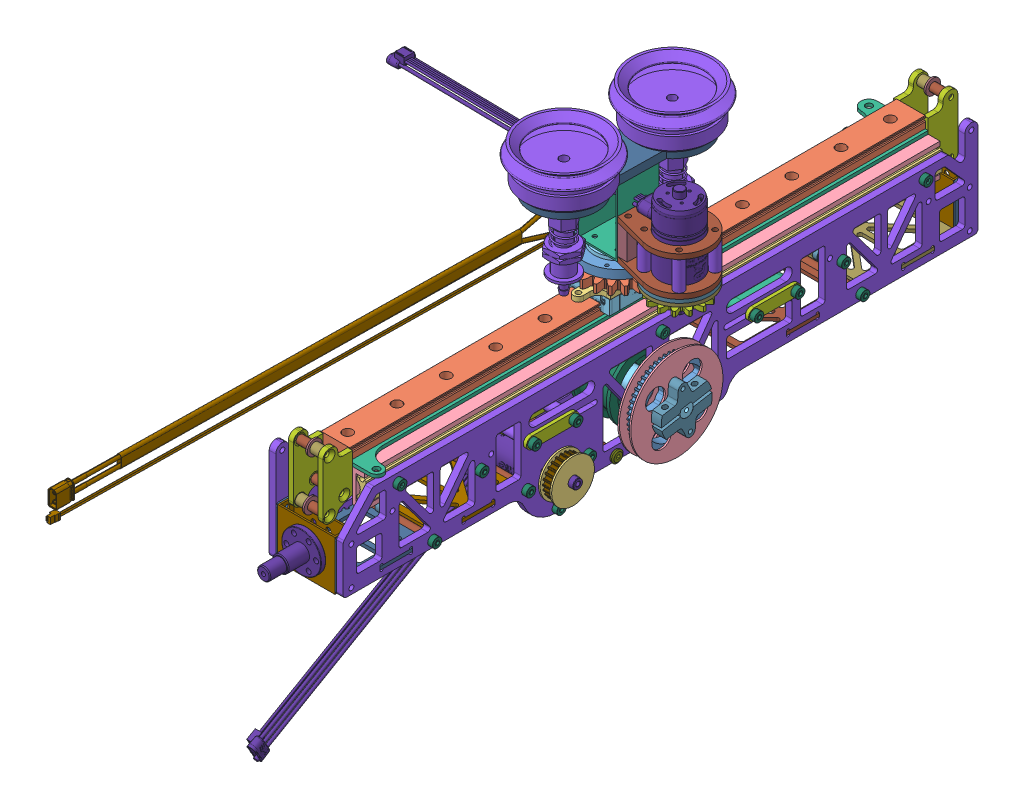
SolidWorks assembly 取矿横移总装, configuration 默认. Lengths in mm.
Overall size (203.34 276.76 526.28).
149 component instances, 51 part files, 3 mates.
Components (placement in the parent):
- 横移总装2.0-1: 横移总装2.0 [默认] at origin size (67.7 199.63 415.26)
  - 20x20x1铝方管-1: 20x20x1铝方管 [默认] at (0 2.5 0.2898) size (15 15 350)
  - 上银直线导轨线性滑轨MGW-C╱MGW-H[MGW9C2R355EZACHCI]_2-1: 上银直线导轨线性滑轨MGW-C╱MGW-H[MGW9C2R355EZACHCI]_2 [横移] at (0 14.9 0.2898) size (18 7 350)
  - 铝合金抽屉滑轨_350-1: 铝合金抽屉滑轨_350 [默认] at (12.9 0 0) x (0 0 -1) z (-1 0 0) size (350.29 20 8) (flexible)
    - 铝合金抽屉滑轨内侧_350-1: 铝合金抽屉滑轨内侧_350 [默认] at origin size (350 12 5.6)
    - 铝合金抽屉滑轨外侧_350-1: 铝合金抽屉滑轨外侧_350 [默认] at (-0.2898 0 2.4) size (350 20 7.2)
  - 铝合金抽屉滑轨_350-2: 铝合金抽屉滑轨_350 [默认] at (-12.9 0 0) x (0 0 -1) z (1 0 0) size (350.29 20 8) (flexible)
    - 铝合金抽屉滑轨内侧_350-1: 铝合金抽屉滑轨内侧_350 [默认] at origin size (350 12 5.6)
    - 铝合金抽屉滑轨外侧_350-1: 铝合金抽屉滑轨外侧_350 [默认] at (-0.2898 0 2.4) size (350 20 7.2)
  - 上银直线导轨线性滑轨MGW-C╱MGW-H[MGW9C2R355EZACHCI]_1-1: 上银直线导轨线性滑轨MGW-C╱MGW-H[MGW9C2R355EZACHCI]_1 [MGW9C] at (0 14.9 3.3555) size (30 9.1 39.49)
  - 滑轨安装板-1: 滑轨安装板 [默认] at (0 10 0.2898) x (0 0 -1) z (0 1 0) size (350 50.5 2)
  - 转点安装板1-1: 转点安装板1 [默认] at (7.5 2.5 160.2898) x (0 0 -1) z (1 0 0) size (48 39.5 3)
  - 转点安装板1-2: 转点安装板1 [默认] at (-10.5 2.5 160.2898) x (0 0 -1) z (1 0 0) size (48 39.5 3)
  - 转点安装板1-3: 转点安装板1 [默认] at (10.5 2.5 -159.7102) x (0 0 1) z (-1 0 0) size (48 39.5 3)
  - 转点安装板1-4: 转点安装板1 [默认] at (-7.5 2.5 -159.7102) x (0 0 1) z (-1 0 0) size (48 39.5 3)
  - 安装固定板-2: 安装固定板 [非2006安装板] at (-22.5 -20 0) x (0 0 -1) z (1 0 0) size (386 79.31 4)
  - 35x10x1铝方管-1: 35x10x1铝方管 [默认] at (0 -30 188) x (1 0 0) z (0 -1 0) size (35 10 30)
  - 垫板-1: 垫板 [默认] at (-18 -30 188) x (0 0 1) z (-1 0 0) size (10 30 1)
  - 垫板-2: 垫板 [默认] at (18 -30 188) x (0 0 1) z (-1 0 0) size (10 30 1)
  - 35x10x1铝方管-2: 35x10x1铝方管 [默认] at (0 -30 -188) x (1 0 0) z (0 -1 0) size (35 10 30)
  - 垫板-3: 垫板 [默认] at (-18 -30 -188) x (0 0 1) z (-1 0 0) size (10 30 1)
  - 垫板-4: 垫板 [默认] at (18 -30 -188) x (0 0 1) z (-1 0 0) size (10 30 1)
  - 鸿康明铝柱-1: 鸿康明铝柱 [M3*8] at (-3.5 22.5 189.2898) x (1 0 0) z (0 -0.954265 0.298963) size (8 5 5)
  - 粉末冶金铜套-1: 粉末冶金铜套 [默认] at (4.5 22.5 189.2898) x (0 0.169784 0.985481) z (-1 0 0) size (6 6 6)
  - 3x9x1垫片-1: 3x9x1垫片 [默认] at (1 22.5 189.2898) x (0 -0.61264 -0.790362) z (1 0 0) size (9 9 1)
  - 鸿康明铝柱-2: 鸿康明铝柱 [M3*8] at (-3.5 -2.5 180.2898) x (1 0 0) z (0 -0.617564 0.786521) size (8 5 5)
  - 粉末冶金铜套-2: 粉末冶金铜套 [默认] at (4.5 -2.5 180.2898) x (0 -0.015386 0.999882) z (-1 0 0) size (6 6 6)
  - 3x9x1垫片-2: 3x9x1垫片 [默认] at (1 -2.5 180.2898) x (0 -0.61264 -0.790362) z (1 0 0) size (9 9 1)
  - 粉末冶金铜套-3: 粉末冶金铜套 [默认] at (-4.5 -9 189.2898) x (0 -0.015317 0.999883) z (-1 0 0) size (6 6 6)
  - 鸿康明铝柱-3: 鸿康明铝柱 [M3*8] at (3.5 -9 189.2898) x (1 0 0) z (0 -0.94021 0.340594) size (8 5 5)
  - 3x9x1垫片-3: 3x9x1垫片 [默认] at (-1 -9 189.2898) x (0 -0.634328 -0.773064) z (1 0 0) size (9 9 1)
  - 鸿康明铝柱-4: 鸿康明铝柱 [M3*8] at (3.5 22.5 -188.7102) x (1 0 0) z (0 -0.954265 0.298963) size (8 5 5)
  - 粉末冶金铜套-4: 粉末冶金铜套 [默认] at (-4.5 22.5 -188.7102) x (0 0.169784 0.985481) z (-1 0 0) size (6 6 6)
  - 3x9x1垫片-4: 3x9x1垫片 [默认] at (-1 22.5 -188.7102) x (0 -0.708763 -0.705447) z (1 0 0) size (9 9 1)
  - 鸿康明铝柱-5: 鸿康明铝柱 [M3*8] at (3.5 -2.5 -179.7102) x (1 0 0) z (0 -0.919061 0.394116) size (8 5 5)
  - 粉末冶金铜套-5: 粉末冶金铜套 [默认] at (-4.5 -2.5 -179.7102) x (0 0.138586 0.99035) z (-1 0 0) size (6 6 6)
  - 3x9x1垫片-5: 3x9x1垫片 [默认] at (-1 -2.5 -179.7102) x (0 -0.708763 -0.705447) z (1 0 0) size (9 9 1)
  - 鸿康明铝柱-6: 鸿康明铝柱 [M3*8] at (-3.5 -9 -188.7102) x (1 0 0) z (0 -0.453676 0.891166) size (8 5 5)
  - 3x9x1垫片-6: 3x9x1垫片 [默认] at (1 -9 -188.7102) x (0 -0.708763 -0.705447) z (1 0 0) size (9 9 1)
  - 粉末冶金铜套-6: 粉末冶金铜套 [默认] at (4.5 -9 -188.7102) x (0 0.138586 0.99035) z (-1 0 0) size (6 6 6)
  - 深沟球轴承-1: 深沟球轴承 [3x7x3] at (15.2 -13.5 163) x (0 -0.844681 -0.53527) z (0 -0.53527 0.844681) size (7 3 7)
  - 深沟球轴承-2: 深沟球轴承 [3x7x3] at (15.2 0.4813 104.6517) x (0 -0.771668 0.636026) z (0 0.636026 0.771668) size (7 3 7)
  - 深沟球轴承-3: 深沟球轴承 [3x7x3] at (15.2 -13.5 -103) x (0 -0.533975 -0.845501) z (0 -0.845501 0.533975) size (7 3 7)
  - 深沟球轴承-4: 深沟球轴承 [3x7x3] at (15.2 -13.5 -163) x (0 0.004458 -0.99999) z (0 -0.99999 -0.004458) size (7 3 7)
  - 深沟球轴承-5: 深沟球轴承 [3x7x3] at (-18.2 -13.5 163) x (0 -0.963854 -0.266431) z (0 -0.266431 0.963854) size (7 3 7)
  - 深沟球轴承-6: 深沟球轴承 [3x7x3] at (-18.2 -13.5 103) x (0 0.996588 0.082533) z (0 0.082533 -0.996588) size (7 3 7)
  - 深沟球轴承-7: 深沟球轴承 [3x7x3] at (-18.2 -13.5 -103) x (0 -0.057804 -0.998328) z (0 -0.998328 0.057804) size (7 3 7)
  - 深沟球轴承-8: 深沟球轴承 [3x7x3] at (-18.2 -13.5 -163) x (0 -0.915157 -0.403098) z (0 -0.403098 0.915157) size (7 3 7)
  - 铰轮1.0-1: 铰轮1.0 [默认] at (0 -34 0) x (0 0.984367 0.176128) z (0 -0.176128 0.984367) size (41 24 41)
  - 法兰轴承-1: 法兰轴承 [10*19*5-1] at (17.5 -34 0) x (0 -0.704143 0.710058) z (0 0.710058 0.704143) size (21 5 21)
  - RoboMaster M2006 P36直流无刷减速电机-1: RoboMaster M2006 P36直流无刷减速电机 [默认] at (-11.3952 -31.5927 46.0167) x (0 -0.258819 -0.965926) z (-1 0 0) size (140.17 141.41 64.8)
  - 安装固定板-3: 安装固定板 [2006安装板] at (18.5 -20 0) x (0 0 -1) z (1 0 0) size (386 79.31 4)
  - 小带轮3Mx25-1: 小带轮3Mx25 [默认] at (25.4 -42.8 63.1397) x (1 0 0) z (0 -0.934457 -0.356076) size (6 23.05 23.09)
  - 大带轮3Mx50-1: 大带轮3Mx50 [默认] at (25.4 -34 0) x (1 0 0) z (0 0.986511 0.163695) size (6 46.93 46.99)
  - 推力球轴承-1: 推力球轴承 [F6-12M 6*12*4] at (24.4 -42.8 63.1397) x (0 0.637207 0.770693) z (0 -0.770693 0.637207) size (12 4 12)
  - 小带轮挡边-1: 小带轮挡边 [默认] at (25.4 -42.8 63.1397) x (0 0.491726 0.87075) z (-1 0 0) size (26 26 1)
  - 小带轮挡边-2: 小带轮挡边 [默认] at (32.4 -42.8 63.1397) x (0 0.997033 0.076981) z (-1 0 0) size (26 26 1)
  - 大带轮挡边-1: 大带轮挡边 [默认] at (32.4 -34 0) x (0 -0.163695 0.986511) z (-1 0 0) size (56 56 1)
  - 大带轮挡边-2: 大带轮挡边 [默认] at (25.4 -34 0) x (0 -0.163695 0.986511) z (-1 0 0) size (56 56 1)
  - 法兰轴承-2: 法兰轴承 [10*19*5-1] at (-17.5 -34 0) x (0 0.968123 0.250476) z (0 -0.250476 0.968123) size (21 5 21)
  - 传动轴-1: 传动轴 [默认] at (-22.5 -34 0) x (0 -0.984367 -0.176128) z (-1 0 0) size (24 24 60.8)
  - 鸿康明铝柱-7: 鸿康明铝柱 [M3*37] at (0 -18 110) size (37 5 5)
  - 鸿康明铝柱-8: 鸿康明铝柱 [M3*37] at (0 -18 -110) size (37 5 5)
  - 槽轮安装件-1: 槽轮安装件 [默认] at (-5 -18 67.5) x (0 0 1) z (0 1 0) size (32 23 7)
  - 槽轮安装件-2: 槽轮安装件 [默认] at (5 -18 -67.5) x (0 0 -1) z (0 1 0) size (32 23 7)
  - 垫片安装-1: 垫片安装 [默认] at (17.5 -18 -67.5) x (0 0 -1) z (1 0 0) size (32 7 2)
  - 垫片安装-2: 垫片安装 [默认] at (-7.5 -18 -67.5) x (0 0 -1) z (1 0 0) size (32 7 2)
  - 垫片安装-3: 垫片安装 [默认] at (-23.5 -18 -67.5) x (0 0 -1) z (1 0 0) size (32 7 2)
  - 304不锈钢接线柱-1: 304不锈钢接线柱 [M3*10-6] at (-13.5 -18 -80) x (0 0.392513 0.919746) z (-1 0 0) size (6 6 10)
  - 304不锈钢接线柱-2: 304不锈钢接线柱 [M3*10-6] at (-13.5 -18 -55) x (0 0.520007 0.854162) z (-1 0 0) size (6 6 10)
  - 垫片安装-4: 垫片安装 [默认] at (23.5 -18 -67.5) x (0 0 -1) z (1 0 0) size (32 7 2)
  - 垫片安装-5: 垫片安装 [默认] at (-17.5 -18 67.5) x (0 0 -1) z (1 0 0) size (32 7 2)
  - 垫片安装-6: 垫片安装 [默认] at (7.5 -18 67.5) x (0 0 -1) z (1 0 0) size (32 7 2)
  - 垫片安装-7: 垫片安装 [默认] at (23.5 -18 67.5) x (0 0 -1) z (1 0 0) size (32 7 2)
  - 垫片安装-8: 垫片安装 [默认] at (-23.5 -18 67.5) x (0 0 -1) z (1 0 0) size (32 7 2)
  - 304不锈钢接线柱-3: 304不锈钢接线柱 [M3*10-6] at (13.5 -18 80) x (0 0.51626 0.856432) z (-1 0 0) size (6 6 10)
  - 304不锈钢接线柱-4: 304不锈钢接线柱 [M3*10-6] at (13.5 -18 55) x (0 0.48843 0.872603) z (-1 0 0) size (6 6 10)
  - 鸿康明铝柱-9: 鸿康明铝柱 [M3*37] at (0 -41 138.7695) size (37 5 5)
  - 鸿康明铝柱-10: 鸿康明铝柱 [M3*37] at (0 -42.8 81.6519) size (37 5 5)
  - 鸿康明铝柱-11: 鸿康明铝柱 [M3*37] at (0 -61.3122 63.1397) size (37 5 5)
  - 鸿康明铝柱-12: 鸿康明铝柱 [M3*37] at (0 -42.8 44.6275) size (37 5 5)
  - 鸿康明铝柱-13: 鸿康明铝柱 [M3*37] at (0 -52 27.5) size (37 5 5)
  - 鸿康明铝柱-14: 鸿康明铝柱 [M3*37] at (0 -52 -27.5) size (37 5 5)
  - 鸿康明铝柱-16: 鸿康明铝柱 [M3*37] at (0 -41 -121.5) x (1 0 0) z (0 -0.672533 0.740067) size (37 5 5)
  - 加强板1-1: 加强板1 [默认] at (0 -39 110.5695) x (0 0 -1) z (0 -1 0) size (50 45 2)
  - 加强板2-1: 加强板2 [默认] at (0 -41 161.9695) x (1 0 0) z (0 1 0) size (45 40 2)
  - 加强板3-1: 加强板3 [默认] at (0 -41 -85.8) x (0 0 1) z (-1 0 0) size (65 2 45)
  - 加强板4-1: 加强板4 [默认] at (0 -41 -153.2) x (0 0 1) z (-1 0 0) size (57 2 45)
  - 2006D型孔联轴器-1: 2006D型孔联轴器 [默认] at (35.4 -42.8 63.1397) x (0 0.844273 0.535914) z (-1 0 0) size (19.05 22 6) (hidden)
  - V型轴承623zz-1: V型轴承623zz [默认] at (4 -18 55) x (1 0 0) z (0 -0.119134 0.992878) size (3.8 12 12)
  - V型轴承623zz-2: V型轴承623zz [默认] at (-4 -18 -55) x (1 0 0) z (0 -0.119134 0.992878) size (3.8 12 12)
  - 夹紧连轴器-1: 夹紧连轴器 [默认] at (35.4 -34 0) x (0 0.176128 -0.984367) z (1 0 0) size (30.94 31 6)
  - 12.9级圆柱头螺钉-1: 12.9级圆柱头螺钉 [M3*10] at (25.5 -41 138.7695) x (0 -0.265301 -0.964166) z (1 0 0) size (5.68 5.68 13)
  - 12.9级圆柱头螺钉-2: 12.9级圆柱头螺钉 [M3*10] at (25.5 -18 110) x (0 -0.265301 -0.964166) z (1 0 0) size (5.68 5.68 13)
  - 12.9级圆柱头螺钉-3: 12.9级圆柱头螺钉 [M3*10] at (25.5 -42.8 81.6519) x (0 -0.265301 -0.964166) z (1 0 0) size (5.68 5.68 13)
  - 12.9级圆柱头螺钉-4: 12.9级圆柱头螺钉 [M3*10] at (27.5 -18 80) x (0 -0.265301 -0.964166) z (1 0 0) size (5.68 5.68 13)
  - 12.9级圆柱头螺钉-5: 12.9级圆柱头螺钉 [M3*10] at (27.5 -18 55) x (0 -0.265301 -0.964166) z (1 0 0) size (5.68 5.68 13)
  - 12.9级圆柱头螺钉-6: 12.9级圆柱头螺钉 [M3*10] at (25.5 -61.3122 63.1397) x (0 -0.265301 -0.964166) z (1 0 0) size (5.68 5.68 13)
  - 12.9级圆柱头螺钉-8: 12.9级圆柱头螺钉 [M3*10] at (25.5 -52 -27.5) x (0 -0.265301 -0.964166) z (1 0 0) size (5.68 5.68 13)
  - 12.9级圆柱头螺钉-9: 12.9级圆柱头螺钉 [M3*10] at (27.5 -18 -55) x (0 -0.265301 -0.964166) z (1 0 0) size (5.68 5.68 13)
  - 12.9级圆柱头螺钉-10: 12.9级圆柱头螺钉 [M3*10] at (27.5 -18 -80) x (0 -0.265301 -0.964166) z (1 0 0) size (5.68 5.68 13)
  - 12.9级圆柱头螺钉-11: 12.9级圆柱头螺钉 [M3*10] at (25.5 -18 -110) x (0 -0.265301 -0.964166) z (1 0 0) size (5.68 5.68 13)
  - 12.9级圆柱头螺钉-12: 12.9级圆柱头螺钉 [M3*10] at (25.5 -41 -121.5) x (0 -0.265301 -0.964166) z (1 0 0) size (5.68 5.68 13)
  - 12.9级圆柱头螺钉-13: 12.9级圆柱头螺钉 [M3*10] at (-25.5 -41 -121.5) x (0 -0.999995 -0.003259) z (-1 0 0) size (5.68 5.68 13)
  - 12.9级圆柱头螺钉-14: 12.9级圆柱头螺钉 [M3*10] at (-25.5 -18 -110) x (0 -0.999995 -0.003259) z (-1 0 0) size (5.68 5.68 13)
  - 12.9级圆柱头螺钉-15: 12.9级圆柱头螺钉 [M3*10] at (-27.5 -18 -80) x (0 -0.999995 -0.003259) z (-1 0 0) size (5.68 5.68 13)
  - 12.9级圆柱头螺钉-16: 12.9级圆柱头螺钉 [M3*10] at (-27.5 -18 -55) x (0 -0.999995 -0.003259) z (-1 0 0) size (5.68 5.68 13)
  - 12.9级圆柱头螺钉-17: 12.9级圆柱头螺钉 [M3*10] at (-25.5 -52 -27.5) x (0 -0.999995 -0.003259) z (-1 0 0) size (5.68 5.68 13)
  - 12.9级圆柱头螺钉-18: 12.9级圆柱头螺钉 [M3*10] at (-25.5 -52 27.5) x (0 -0.999995 -0.003259) z (-1 0 0) size (5.68 5.68 13)
  - 12.9级圆柱头螺钉-19: 12.9级圆柱头螺钉 [M3*10] at (-25.5 -42.8 44.6275) x (0 -0.999995 -0.003259) z (-1 0 0) size (5.68 5.68 13)
  - 12.9级圆柱头螺钉-20: 12.9级圆柱头螺钉 [M3*10] at (-27.5 -18 55) x (0 -0.999995 -0.003259) z (-1 0 0) size (5.68 5.68 13)
  - 12.9级圆柱头螺钉-21: 12.9级圆柱头螺钉 [M3*10] at (-27.5 -18 80) x (0 -0.999995 -0.003259) z (-1 0 0) size (5.68 5.68 13)
  - 12.9级圆柱头螺钉-22: 12.9级圆柱头螺钉 [M3*10] at (-25.5 -61.3122 63.1397) x (0 -0.999995 -0.003259) z (-1 0 0) size (5.68 5.68 13)
  - 12.9级圆柱头螺钉-23: 12.9级圆柱头螺钉 [M3*10] at (-25.5 -42.8 81.6519) x (0 -0.999995 -0.003259) z (-1 0 0) size (5.68 5.68 13)
  - 12.9级圆柱头螺钉-24: 12.9级圆柱头螺钉 [M3*10] at (-25.5 -18 110) x (0 -0.999995 -0.003259) z (-1 0 0) size (5.68 5.68 13)
  - 12.9级圆柱头螺钉-25: 12.9级圆柱头螺钉 [M3*10] at (-25.5 -41 138.7695) x (0 -0.999995 -0.003259) z (-1 0 0) size (5.68 5.68 13)
  - 12.9级圆柱头螺钉-26: 12.9级圆柱头螺钉 [M3*8] at (-25.5 0 160) x (0 -0.999995 -0.003259) z (-1 0 0) size (5.68 5.68 11)
  - 12.9级圆柱头螺钉-27: 12.9级圆柱头螺钉 [M3*8] at (-25.5 0 0) x (0 -0.999995 -0.003259) z (-1 0 0) size (5.68 5.68 11)
  - 12.9级圆柱头螺钉-28: 12.9级圆柱头螺钉 [M3*8] at (-25.5 0 -160) x (0 -0.999995 -0.003259) z (-1 0 0) size (5.68 5.68 11)
  - 12.9级圆柱头螺钉-29: 12.9级圆柱头螺钉 [M3*8] at (25.5 0 -160) x (0 -0.774925 -0.632053) z (1 0 0) size (5.68 5.68 11)
  - 12.9级圆柱头螺钉-30: 12.9级圆柱头螺钉 [M3*8] at (25.5 0 0) x (0 -0.774925 -0.632053) z (1 0 0) size (5.68 5.68 11)
  - 12.9级圆柱头螺钉-31: 12.9级圆柱头螺钉 [M3*8] at (25.5 0 160) x (0 -0.774925 -0.632053) z (1 0 0) size (5.68 5.68 11)
  - 304不锈钢平头倒边螺丝-1: 304不锈钢平头倒边螺丝 [M3*10] at (24.3 -52 27.5) x (0 0.904522 -0.426427) z (1 0 0) size (7 7 11.8)
  - 12.9级圆柱头螺钉-32: 12.9级圆柱头螺钉 [M3*10] at (25.5 -42.8 44.6275) x (0 -0.265301 -0.964166) z (1 0 0) size (5.68 5.68 13)
  - 转点法兰-1: 转点法兰 [默认] at (0 -30 193) x (0.866025 0.5 0) z (0 0 1) size (24 24 26)
- 吸盘总装-1: 吸盘总装 [默认] at (0 34 3.3555) x (-1 0 0) z (0 1 0) size (203.34 428.51 86.1)
  - 6750zz-1: 6750zz [默认] at origin size (32 32 4)
  - 轴承外圈固定-1: 轴承外圈固定 [默认] at (0 0 0.03) x (0 -1 0) z (0 0 1) size (42 42 5.34)
  - 圆柱齿轮24×2-1: 圆柱齿轮24×2 [默认] at (0 0 -4.5) size (51.72 51.72 5)
  - 拉线安装版-1: 拉线安装版 [默认] at (0 0 -10) x (0 1 0) z (0 0 1) size (63.3 30 3)
  - 内圈分离铝件-1: 内圈分离铝件 [默认] at (0 0 1.95) x (-0.717753 -0.696298 0) z (0 0 -1) size (28 28 5.15)
  - 内圈压板-1: 内圈压板 [默认] at (0 0 2) x (0.717753 0.696298 0) z (0 0 1) size (28 28 3)
  - 20x40x1铝方管-2: 20x40x1铝方管 [默认] at (0 0 25) x (-0.999885 0.015171 0) z (0.015171 0.999885 0) size (25 40 25)
  - RoboMaster M2006 P36直流无刷减速电机-1: RoboMaster M2006 P36直流无刷减速电机 [默认] at (-58.4085 2.0306 32.7952) x (-0.717753 -0.696298 0) z (0 0 1) size (140.17 141.41 64.8)
  - 圆柱齿轮14×2-1: 圆柱齿轮14×2 [默认] at (-37.9956 0.5765 -4.5) x (-0.882361 0.470573 0) z (0 0 1) size (32 31.46 3)
  - 推力球轴承-1: 推力球轴承 [F6-12M 6*12*4] at (-37.9956 0.5765 -3) x (0.191226 -0.981546 0) z (-0.981546 -0.191226 0) size (12 4 12)
  - 吸盘-1: 吸盘 [PJTS-50-6-N] at (-0.493 -32.4963 72) x (-0.999885 0.015171 0) z (-0.015171 -0.999885 0) size (54.83 80 54.83)
  - 吸盘-2: 吸盘 [PJTS-50-6-N] at (0.493 32.4963 72) x (0.996645 0.081841 0) z (-0.081841 0.996645 0) size (54.83 80 54.83)
  - C610无刷电机调速器-1: C610无刷电机调速器 [默认] at (16.0987 6.3023 -120.7197) x (0 0 -1) z (0.999885 -0.015171 0) size (22.14 353.32 7.25)
  - 吸盘固定板2-1: 吸盘固定板2 [默认] at (0 0 45) x (0.015171 0.999885 0) z (0 0 1) size (105 40 5)
  - 2006电机紧固板-1: 2006电机紧固板 [默认] at (-37.9956 0.5765 8) x (0.999885 -0.015171 0) z (0 0 -1) size (43.75 36.5 3)
  - 2006电机安装板-1: 2006电机安装板 [默认] at (-37.9956 0.5765 0.9) x (-0.999885 0.015171 0) z (0 0 1) size (35.09 36.5 2)
  - 2006电机紧固板-2: 2006电机紧固板 [默认] at (-37.9956 0.5765 29) x (0.999885 -0.015171 0) z (0 0 -1) size (43.75 36.5 3)
  - 304不锈钢接线柱-1: 304不锈钢接线柱 [M3*18-6] at (-48.9414 -10.0421 17) size (6 6 18)
  - 304不锈钢接线柱-2: 304不锈钢接线柱 [M3*18-6] at (-48.6142 11.5222 17) x (-0.15981 -0.987148 0) z (0 0 1) size (6 6 18)
  - 304不锈钢接线柱-3: 304不锈钢接线柱 [M3*18-6] at (-27.0499 11.195 17) size (6 6 18)
  - 304不锈钢接线柱-4: 304不锈钢接线柱 [M3*18-6] at (-27.3771 -10.3692 17) size (6 6 18)
  - 安装铝件-1: 安装铝件 [默认] at (-15.4982 0.2351 17) x (-0.015171 -0.999885 0) z (0.999885 -0.015171 0) size (25 18 6)
  - 2006电机安装垫块-1: 2006电机安装垫块 [默认] at (-37.9956 0.5765 3.95) x (-0.999885 0.015171 0) z (0 0 1) size (35.09 36.5 2.1)
Mates (geometry in assembly coordinates):
- 重合1: coincident anti-aligned: plane of 横移总装2.0-1/上银直线导轨线性滑轨MGW-C╱MGW-H[MGW9C2R355EZACHCI]_1-1 through (-15 24 17.1055) normal (0 1 0); plane of 吸盘总装-1/拉线安装版-1 through (0 24 3.3555) normal (0 -1 0)
- 宽度1: width anti-aligned: plane of 吸盘总装-1/拉线安装版-1 through (-15 27 -16.2945) normal (-1 0 0); plane of 吸盘总装-1/拉线安装版-1 through (15 27 -16.2945) normal (1 0 0); plane of 横移总装2.0-1/上银直线导轨线性滑轨MGW-C╱MGW-H[MGW9C2R355EZACHCI]_1-1 through (15 22 17.1055) normal (1 0 0); plane of 横移总装2.0-1/上银直线导轨线性滑轨MGW-C╱MGW-H[MGW9C2R355EZACHCI]_1-1 through (-15 22 17.1055) normal (-1 0 0)
- 宽度2: width aligned: plane of 吸盘总装-1/拉线安装版-1 through (-15 27 -16.2945) normal (0 0 -1); plane of 吸盘总装-1/拉线安装版-1 through (-15 27 23.0055) normal (0 0 1); plane of 横移总装2.0-1/上银直线导轨线性滑轨MGW-C╱MGW-H[MGW9C2R355EZACHCI]_1-1 through (0 0.5867 -16.2945) normal (0 0 -1); plane of 横移总装2.0-1/上银直线导轨线性滑轨MGW-C╱MGW-H[MGW9C2R355EZACHCI]_1-1 through (0 0.5867 23.0055) normal (0 0 1)
